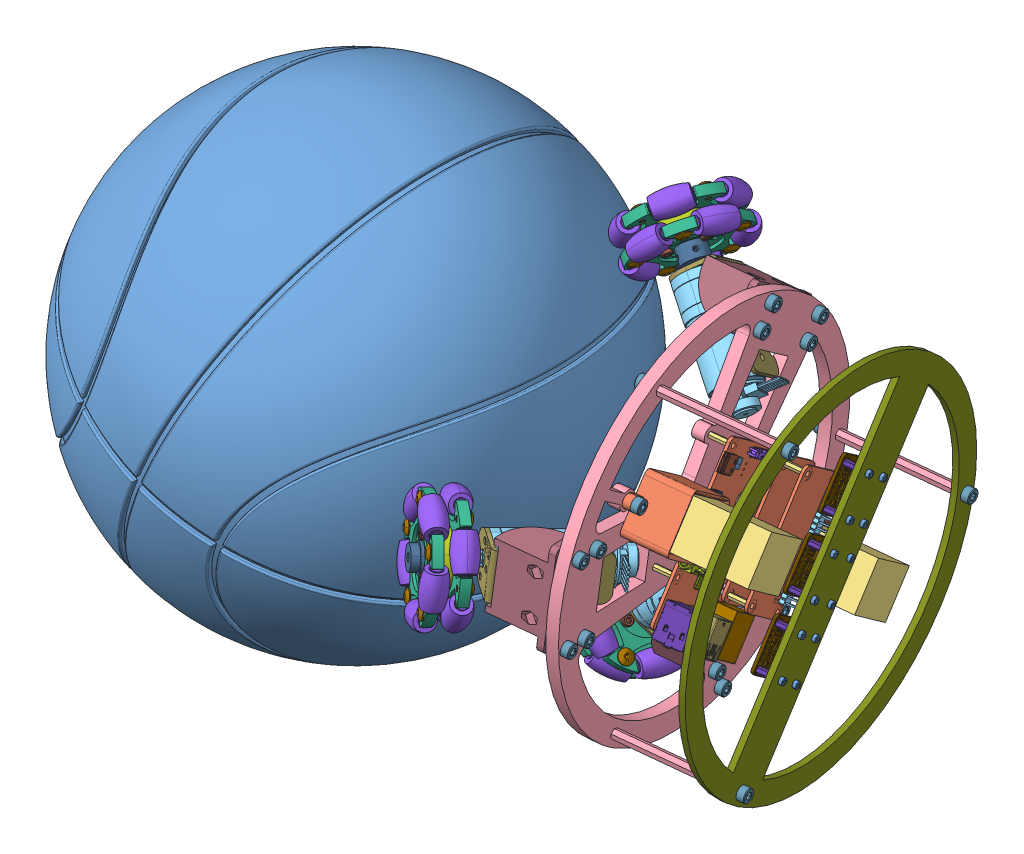
SolidWorks assembly FullAssembly, configuration Default. Lengths in mm.
Overall size (421.56 325.38 301.94).
211 component instances, 40 part files, 36 mates.
Components (placement in the parent):
- basketball-1: basketball [Default] at (262.8236 329.342 181.7922) x (0.927184 -0.374607 0) z (0 0 1) size (249.95 249.95 250.98)
- PiAssembly-1: PiAssembly [Default] at (395.3166 293.6839 90.7968) x (0.056245 -0.796975 0.601388) z (0.155278 0.601995 0.783257) size (89.02 42.68 58.4)
  - Raspberry Pi 4 Model B-1: Raspberry Pi 4 Model B [Default] at (23.6028 37.8671 72.1656) size (88.99 19.9 58.4)
    - PCB, RPi4ModelB-1: PCB, RPi4ModelB [Default] at origin size (85 1.6 56)
    - Broadcom BCM2711B0 CPU, RPi4ModelB-1: Broadcom BCM2711B0 CPU, RPi4ModelB [Default] at (-13.25 0.8 -4.5) size (15 2.3 15)
    - 2.54 mm DUPONT MALE PIN HEADER, POE, 2X2, RPi4ModelB-1: 2.54 mm DUPONT MALE PIN HEADER, POE, 2X2, RPi4ModelB [Default] at (19 0.8 -18.5) size (5.08 11.3 5.08)
    - 2.54 mm DUPONT MALE PIN HEADER, IO, 2X20, RPi4ModelB-1: 2.54 mm DUPONT MALE PIN HEADER, IO, 2X20, RPi4ModelB [Default] at (-10 0.8 -24.5) size (50.8 11.3 5.08)
    - Camera Connector, RPi4ModelB-1: Camera Connector, RPi4ModelB [Default] at (4 0.8 16.5) x (0 0 -1) z (1 0 0) size (22.4 5.68 5.07)
    - Microphone Plug, RPi4ModelB-1: Microphone Plug, RPi4ModelB [Default] at (11.5 0.8 21.65) size (7.23 7.55 15)
    - Display Connector, RPi4ModelB-1: Display Connector, RPi4ModelB [Default] at (-38.5 0.8 0) x (0 0 1) z (-1 0 0) size (22.4 5.68 5.07)
    - Gigabit Ethernet Port, RPi4ModelB-1: Gigabit Ethernet Port, RPi4ModelB [Default] at (45.5 7.55 -17.75) x (0 0 -1) z (1 0 0) size (16.2 17.24 21.64)
    - Female Micro HDMI Connector, RPi4ModelB-2: Female Micro HDMI Connector, RPi4ModelB [Default] at (-3 0.8 27.3875) size (6.5 3.51 7.5)
    - Female Micro HDMI Connector, RPi4ModelB-3: Female Micro HDMI Connector, RPi4ModelB [Default] at (-16.5 0.8 27.3875) size (6.5 3.51 7.5)
    - Female USB Type C Connector, RPi4ModelB-1: Female USB Type C Connector, RPi4ModelB [Default] at (-31.3 0.8 26.5419) size (8.94 3.96 7.9)
    - 2X USB3.0 PORTS, RPi4ModelB-2: 2X USB3.0 PORTS, RPi4ModelB [Default] at (37.07 0.8 1) size (17.47 19.41 15.68)
    - 91D77 D9WHV 778K, 4 GB LPDDR4 SDRAM, RPi4ModelB-1: 91D77 D9WHV 778K, 4 GB LPDDR4 SDRAM, RPi4ModelB [Default] at (2.25 0.8 -4.5) size (10 0.8 14.5)
    - Cypress CYW43455 Wireless Module Cover, RPi4ModelB-1: Cypress CYW43455 Wireless Module Cover, RPi4ModelB [Default] at (-30.5 0.8 -14.5) size (11 1.6 13)
    - SD Card Slot, RPi4ModelB-1: SD Card Slot, RPi4ModelB [Default] at (-35.3 -0.8 0) x (0 0 -1) z (-1 0 0) size (11.95 1.45 11.4)
    - VIA VL805 PCIe USB 3.0 controller, RPi4ModelB-1: VIA VL805 PCIe USB 3.0 controller, RPi4ModelB [Default] at (17.5 0.8 4) size (8.8 0.8 8.8)
    - 2X USB2.0 PORTS, RPi4ModelB-1: 2X USB2.0 PORTS, RPi4ModelB [Default] at (37.065 0.65 19) size (17.87 19.16 15.33)
    - Broadcom BCM54213PE Gigabit Ethernet Transceiver, RPi4ModelB-1: Broadcom BCM54213PE Gigabit Ethernet Transceiver, RPi4ModelB [Default] at (16.5 0.8 -10) size (6.8 1 6.8)
    - MxL7704 Universal PMIC, RPi4ModelB-1: MxL7704 Universal PMIC, RPi4ModelB [Default] at (-32.5 0.8 16) size (5.4 0.8 5.4)
  - Pi Motor Hat-1: Pi Motor Hat [Default] at (13.5778 60.0571 59.1906) size (65 1.5 30)
  - Pi Motor Hat-2: Pi Motor Hat [Default] at (13.5778 48.6571 59.1906) size (65 1.5 30)
  - PiStandoff-1: PiStandoff [Default] at (42.6028 50.0571 47.6656) x (0.096997 0 0.995285) z (-0.995285 0 0.096997) size (3.12 10 2.7)
  - PiStandoff-2: PiStandoff [Default] at (-15.3972 38.6571 47.6656) size (3.12 10 2.7)
  - PiStandoff-3: PiStandoff [Default] at (-15.4472 50.0571 47.6656) x (-0.525395 0 0.850858) z (-0.850858 0 -0.525395) size (3.12 10 2.7)
  - PiStandoff-4: PiStandoff [Default] at (42.6028 38.6571 47.6656) size (3.12 10 2.7)
  - PiStandoff-5: PiStandoff [Default] at (42.6028 50.0571 70.7156) x (0.1639 0 0.986477) z (-0.986477 0 0.1639) size (3.12 10 2.7)
  - PiStandoff-6: PiStandoff [Default] at (-15.4472 50.0571 70.7156) x (-0.245329 0 -0.96944) z (0.96944 0 -0.245329) size (3.12 10 2.7)
  - 2.54 mm DUPONT MALE PIN HEADER, IO, 2X20, RPi4ModelB-1: 2.54 mm DUPONT MALE PIN HEADER, IO, 2X20, RPi4ModelB [Default] at (13.6028 50.0571 47.6656) size (50.8 11.3 5.08)
  - 2.54 mm DUPONT MALE PIN HEADER, IO, 2X20, RPi4ModelB-2: 2.54 mm DUPONT MALE PIN HEADER, IO, 2X20, RPi4ModelB [Default] at (13.6028 61.4571 47.6656) size (50.8 11.3 5.08)
  - PiStandoff-7: PiStandoff [Default] at (42.6028 27.0771 47.6656) x (0.455658 0 0.890155) z (-0.890155 0 0.455658) size (3.12 10 2.7)
  - PiStandoff-8: PiStandoff [Default] at (-15.3972 27.0771 47.6656) x (-0.990783 0 0.135462) z (-0.135462 0 -0.990783) size (3.12 10 2.7)
  - PiStandoff-9: PiStandoff [Default] at (42.6028 27.0771 96.6656) x (0.096997 0 0.995285) z (-0.995285 0 0.096997) size (3.12 10 2.7)
  - PiStandoff-10: PiStandoff [Default] at (-15.3972 27.0771 96.6656) x (0.096997 0 0.995285) z (-0.995285 0 0.096997) size (3.12 10 2.7)
- BasePlate-1: BasePlate [Default] at (428.0251 321.0796 155.392) x (-0.155278 -0.601995 -0.783257) z (0.056245 -0.796975 0.601388) size (200 6.35 200)
- MotorAssembly-1: MotorAssembly [Default] at (403.3898 268.0903 115.0409) x (-0.126349 0.389203 -0.912445) z (-0.772599 -0.615538 -0.155574) size (87.54 86.92 94.1)
  - 25d-metal-gearmotor-20.4-encoder-1: 25d-metal-gearmotor-20.4-encoder [Default] at (-50.1822 -0.1991 13.7812) size (25 32.85 74)
  - WheelAsm-1: WheelAsm [Default] at (-21.6001 -5.321 -11.7274) x (0.801126 0.598496 0) z (0 0 1) size (63.86 60.79 27.6)
    - WheelAsm.STEP-1: WheelAsm.STEP [Default] at origin size (63.86 60.79 27.6)
      - WheelBase.STEP-1: WheelBase.STEP [Default] at (4.9023 2.731 55.3836) x (1 0 0) z (0 -1 0) size (56.86 5 54.96)
      - BasePlacer.STEP-1: BasePlacer.STEP [Default] at (4.9023 2.731 58.8836) x (1 0 0) z (0 -1 0) size (28 10 28)
      - RubberWheel.STEP-1: RubberWheel.STEP [Default] at (4.9023 26.7901 57.8836) x (1 0 0) z (0 -0.999594 -0.028494) size (19 12.5 12.5)
      - RubberWheel.STEP-2: RubberWheel.STEP [Default] at (-17.9792 10.1657 57.8836) x (0.309017 0.951057 0) z (0.95067 -0.308892 -0.028494) size (19 12.5 12.5)
      - RubberWheel.STEP-3: RubberWheel.STEP [Default] at (-9.2392 -16.7332 57.8836) x (-0.809017 0.587785 0) z (0.587547 0.808689 -0.028494) size (19 12.5 12.5)
      - RubberWheel.STEP-4: RubberWheel.STEP [Default] at (19.0439 -16.7332 57.8836) x (-0.809017 -0.587785 0) z (-0.587547 0.808689 -0.028494) size (19 12.5 12.5)
      - RubberWheel.STEP-5: RubberWheel.STEP [Default] at (27.7839 10.1657 57.8836) x (0.309017 -0.951057 0) z (-0.95067 -0.308892 -0.028494) size (19 12.5 12.5)
      - Rivet.STEP-1: Rivet.STEP [Default] at (4.9023 -21.269 54.8836) x (1 0 0) z (0 1 0) size (7.46 6.8 7.46)
      - Rivet.STEP-2: Rivet.STEP [Default] at (27.7277 -4.6854 54.8836) x (0.309017 0.951057 0) z (-0.951057 0.309017 0) size (7.46 6.8 7.46)
      - Rivet.STEP-3: Rivet.STEP [Default] at (19.0092 22.1474 54.8836) x (-0.809017 0.587785 0) z (-0.587785 -0.809017 0) size (7.46 6.8 7.46)
      - Rivet.STEP-4: Rivet.STEP [Default] at (-9.2045 22.1474 54.8836) x (-0.809017 -0.587785 0) z (0.587785 -0.809017 0) size (7.46 6.8 7.46)
      - Rivet.STEP-5: Rivet.STEP [Default] at (-17.923 -4.6854 54.8836) x (0.309017 -0.951057 0) z (0.951057 0.309017 0) size (7.46 6.8 7.46)
      - WheelBase.STEP-2: WheelBase.STEP [Default] at (4.9023 2.731 67.3836) x (-1 0 0) z (0 1 0) size (56.86 5 54.96)
      - RubberWheel.STEP-6: RubberWheel.STEP [Default] at (4.9023 -21.3281 69.8836) size (19 12.5 12.5)
      - RubberWheel.STEP-7: RubberWheel.STEP [Default] at (27.7839 -4.7037 69.8836) x (0.309017 0.951057 0) z (0 0 1) size (19 12.5 12.5)
      - RubberWheel.STEP-8: RubberWheel.STEP [Default] at (19.0439 22.1953 69.8836) x (-0.809017 0.587785 0) z (0 0 1) size (19 12.5 12.5)
      - RubberWheel.STEP-9: RubberWheel.STEP [Default] at (-9.2392 22.1953 69.8836) x (-0.809017 -0.587785 0) z (0 0 1) size (19 12.5 12.5)
      - RubberWheel.STEP-10: RubberWheel.STEP [Default] at (-17.9792 -4.7037 69.8836) x (0.309017 -0.951057 0) z (0 0 1) size (19 12.5 12.5)
      - Rivet.STEP-6: Rivet.STEP [Default] at (-9.2045 -16.6854 72.8836) x (-0.985624 0.168955 0) z (0.168955 0.985624 0) size (7.46 6.8 7.46)
      - Rivet.STEP-7: Rivet.STEP [Default] at (19.0092 -16.6854 72.8836) x (-0.46526 -0.885174 0) z (-0.885174 0.46526 0) size (7.46 6.8 7.46)
      - Rivet.STEP-8: Rivet.STEP [Default] at (27.7277 10.1474 72.8836) x (0.698077 -0.716022 0) z (-0.716022 -0.698077 0) size (7.46 6.8 7.46)
      - Rivet.STEP-9: Rivet.STEP [Default] at (4.9023 26.731 72.8836) x (0.896695 0.442648 0) z (0.442648 -0.896695 0) size (7.46 6.8 7.46)
      - Rivet.STEP-10: Rivet.STEP [Default] at (-17.923 10.1474 72.8836) x (-0.143889 0.989594 0) z (0.989594 0.143889 0) size (7.46 6.8 7.46)
      - ShaftConnector.STEP-1: ShaftConnector.STEP [Default] at (4.9023 2.731 48.8836) x (1 0 0) z (0 -1 0) size (14.01 27.6 14.01)
      - M3HexNut.STEP-1: M3HexNut.STEP [Default] at (13.9956 7.981 72.8836) x (1 0 0) z (0 0 -1) size (5 5 5)
      - M3HexNut.STEP-2: M3HexNut.STEP [Default] at (-4.1909 7.981 72.8836) x (-0.5 0.866025 0) z (0 0 -1) size (5 5 5)
      - M3HexNut.STEP-3: M3HexNut.STEP [Default] at (4.9023 -7.769 72.8836) x (-0.5 -0.866025 0) z (0 0 -1) size (5 5 5)
      - M3HexNut.STEP-4: M3HexNut.STEP [Default] at (4.9023 -7.769 54.8836) size (5 5 5)
      - M3HexNut.STEP-5: M3HexNut.STEP [Default] at (13.9956 7.981 54.8836) x (-0.5 0.866025 0) z (0 0 1) size (5 5 5)
      - M3HexNut.STEP-6: M3HexNut.STEP [Default] at (-4.1909 7.981 54.8836) x (-0.5 -0.866025 0) z (0 0 1) size (5 5 5)
  - pololu-25d-mm-metal-gearmotor-bracket-1: pololu-25d-mm-metal-gearmotor-bracket [Default] at (-20.3072 0.8009 19.6562) x (-1 0 0) z (0 0 1) size (25 27 52)
  - MotorMount-1: MotorMount [Default] at (-1.8072 14.6545 14.1971) x (0 0.707107 0.707107) z (0 -0.707107 0.707107) size (24 50 30)
  - M4x6-1: M4x6 [Default] at (-40.5572 28.337 -7.9707) x (0 -0.707107 0.707107) z (-0.996625 0.05805 0.05805) size (12.15 7 7)
  - M4x6-2: M4x6 [Default] at (-40.5572 36.8223 0.5146) x (0 -0.707107 0.707107) z (-0.996625 0.05805 0.05805) size (12.15 7 7)
  - M3x4-3: M3x4 [Default] at (-8.4572 11.3009 18.2812) x (0 1 0) z (-0.998192 0 -0.0601) size (7 5.5 5.5)
  - M3x4-4: M3x4 [Default] at (-30.1572 11.3009 18.2812) x (0 1 0) z (-0.546944 0 0.837169) size (7 5.5 5.5)
  - M4x6-3: M4x6 [Default] at (1.9428 28.337 -7.9707) x (0 -0.707107 0.707107) z (-0.996625 0.05805 0.05805) size (12.15 7 7)
  - M4x6-4: M4x6 [Default] at (1.9428 36.8223 0.5146) x (0 -0.707107 0.707107) z (-0.996625 0.05805 0.05805) size (12.15 7 7)
- MotorAssembly-2: MotorAssembly [Default] at (412.1642 386.5359 132.8779) x (0.155278 0.601995 0.783257) z (-0.737168 0.598426 -0.313797) size (87.54 86.92 94.1)
  - 25d-metal-gearmotor-20.4-encoder-1: 25d-metal-gearmotor-20.4-encoder [Default] at (-50.1822 -0.1991 13.7812) size (25 32.85 74)
  - WheelAsm-1: WheelAsm [Default] at (-21.6001 -5.321 -11.7274) x (0.801126 0.598496 0) z (0 0 1) size (63.86 60.79 27.6)
    - WheelAsm.STEP-1: WheelAsm.STEP [Default] at origin size (63.86 60.79 27.6)
      - WheelBase.STEP-1: WheelBase.STEP [Default] at (4.9023 2.731 55.3836) x (1 0 0) z (0 -1 0) size (56.86 5 54.96)
      - BasePlacer.STEP-1: BasePlacer.STEP [Default] at (4.9023 2.731 58.8836) x (1 0 0) z (0 -1 0) size (28 10 28)
      - RubberWheel.STEP-1: RubberWheel.STEP [Default] at (4.9023 26.7901 57.8836) x (1 0 0) z (0 -0.999594 -0.028494) size (19 12.5 12.5)
      - RubberWheel.STEP-2: RubberWheel.STEP [Default] at (-17.9792 10.1657 57.8836) x (0.309017 0.951057 0) z (0.95067 -0.308892 -0.028494) size (19 12.5 12.5)
      - RubberWheel.STEP-3: RubberWheel.STEP [Default] at (-9.2392 -16.7332 57.8836) x (-0.809017 0.587785 0) z (0.587547 0.808689 -0.028494) size (19 12.5 12.5)
      - RubberWheel.STEP-4: RubberWheel.STEP [Default] at (19.0439 -16.7332 57.8836) x (-0.809017 -0.587785 0) z (-0.587547 0.808689 -0.028494) size (19 12.5 12.5)
      - RubberWheel.STEP-5: RubberWheel.STEP [Default] at (27.7839 10.1657 57.8836) x (0.309017 -0.951057 0) z (-0.95067 -0.308892 -0.028494) size (19 12.5 12.5)
      - Rivet.STEP-1: Rivet.STEP [Default] at (4.9023 -21.269 54.8836) x (1 0 0) z (0 1 0) size (7.46 6.8 7.46)
      - Rivet.STEP-2: Rivet.STEP [Default] at (27.7277 -4.6854 54.8836) x (0.309017 0.951057 0) z (-0.951057 0.309017 0) size (7.46 6.8 7.46)
      - Rivet.STEP-3: Rivet.STEP [Default] at (19.0092 22.1474 54.8836) x (-0.809017 0.587785 0) z (-0.587785 -0.809017 0) size (7.46 6.8 7.46)
      - Rivet.STEP-4: Rivet.STEP [Default] at (-9.2045 22.1474 54.8836) x (-0.809017 -0.587785 0) z (0.587785 -0.809017 0) size (7.46 6.8 7.46)
      - Rivet.STEP-5: Rivet.STEP [Default] at (-17.923 -4.6854 54.8836) x (0.309017 -0.951057 0) z (0.951057 0.309017 0) size (7.46 6.8 7.46)
      - WheelBase.STEP-2: WheelBase.STEP [Default] at (4.9023 2.731 67.3836) x (-1 0 0) z (0 1 0) size (56.86 5 54.96)
      - RubberWheel.STEP-6: RubberWheel.STEP [Default] at (4.9023 -21.3281 69.8836) size (19 12.5 12.5)
      - RubberWheel.STEP-7: RubberWheel.STEP [Default] at (27.7839 -4.7037 69.8836) x (0.309017 0.951057 0) z (0 0 1) size (19 12.5 12.5)
      - RubberWheel.STEP-8: RubberWheel.STEP [Default] at (19.0439 22.1953 69.8836) x (-0.809017 0.587785 0) z (0 0 1) size (19 12.5 12.5)
      - RubberWheel.STEP-9: RubberWheel.STEP [Default] at (-9.2392 22.1953 69.8836) x (-0.809017 -0.587785 0) z (0 0 1) size (19 12.5 12.5)
      - RubberWheel.STEP-10: RubberWheel.STEP [Default] at (-17.9792 -4.7037 69.8836) x (0.309017 -0.951057 0) z (0 0 1) size (19 12.5 12.5)
      - Rivet.STEP-6: Rivet.STEP [Default] at (-9.2045 -16.6854 72.8836) x (-0.985624 0.168955 0) z (0.168955 0.985624 0) size (7.46 6.8 7.46)
      - Rivet.STEP-7: Rivet.STEP [Default] at (19.0092 -16.6854 72.8836) x (-0.46526 -0.885174 0) z (-0.885174 0.46526 0) size (7.46 6.8 7.46)
      - Rivet.STEP-8: Rivet.STEP [Default] at (27.7277 10.1474 72.8836) x (0.698077 -0.716022 0) z (-0.716022 -0.698077 0) size (7.46 6.8 7.46)
      - Rivet.STEP-9: Rivet.STEP [Default] at (4.9023 26.731 72.8836) x (0.896695 0.442648 0) z (0.442648 -0.896695 0) size (7.46 6.8 7.46)
      - Rivet.STEP-10: Rivet.STEP [Default] at (-17.923 10.1474 72.8836) x (-0.143889 0.989594 0) z (0.989594 0.143889 0) size (7.46 6.8 7.46)
      - ShaftConnector.STEP-1: ShaftConnector.STEP [Default] at (4.9023 2.731 48.8836) x (1 0 0) z (0 -1 0) size (14.01 27.6 14.01)
      - M3HexNut.STEP-1: M3HexNut.STEP [Default] at (13.9956 7.981 72.8836) x (1 0 0) z (0 0 -1) size (5 5 5)
      - M3HexNut.STEP-2: M3HexNut.STEP [Default] at (-4.1909 7.981 72.8836) x (-0.5 0.866025 0) z (0 0 -1) size (5 5 5)
      - M3HexNut.STEP-3: M3HexNut.STEP [Default] at (4.9023 -7.769 72.8836) x (-0.5 -0.866025 0) z (0 0 -1) size (5 5 5)
      - M3HexNut.STEP-4: M3HexNut.STEP [Default] at (4.9023 -7.769 54.8836) size (5 5 5)
      - M3HexNut.STEP-5: M3HexNut.STEP [Default] at (13.9956 7.981 54.8836) x (-0.5 0.866025 0) z (0 0 1) size (5 5 5)
      - M3HexNut.STEP-6: M3HexNut.STEP [Default] at (-4.1909 7.981 54.8836) x (-0.5 -0.866025 0) z (0 0 1) size (5 5 5)
  - pololu-25d-mm-metal-gearmotor-bracket-1: pololu-25d-mm-metal-gearmotor-bracket [Default] at (-20.3072 0.8009 19.6562) x (-1 0 0) z (0 0 1) size (25 27 52)
  - MotorMount-1: MotorMount [Default] at (-1.8072 14.6545 14.1971) x (0 0.707107 0.707107) z (0 -0.707107 0.707107) size (24 50 30)
  - M4x6-1: M4x6 [Default] at (-40.5572 28.337 -7.9707) x (0 -0.707107 0.707107) z (-0.996625 0.05805 0.05805) size (12.15 7 7)
  - M4x6-2: M4x6 [Default] at (-40.5572 36.8223 0.5146) x (0 -0.707107 0.707107) z (-0.996625 0.05805 0.05805) size (12.15 7 7)
  - M3x4-3: M3x4 [Default] at (-8.4572 11.3009 18.2812) x (0 1 0) z (-0.998192 0 -0.0601) size (7 5.5 5.5)
  - M3x4-4: M3x4 [Default] at (-30.1572 11.3009 18.2812) x (0 1 0) z (-0.546944 0 0.837169) size (7 5.5 5.5)
  - M4x6-3: M4x6 [Default] at (1.9428 28.337 -7.9707) x (0 -0.707107 0.707107) z (-0.996625 0.05805 0.05805) size (12.15 7 7)
  - M4x6-4: M4x6 [Default] at (1.9428 36.8223 0.5146) x (0 -0.707107 0.707107) z (-0.996625 0.05805 0.05805) size (12.15 7 7)
- MotorAssembly-3: MotorAssembly [Default] at (423.1824 310.8802 225.5027) x (-0.028929 -0.991198 0.129189) z (-0.582424 0.121751 0.803716) size (87.54 86.92 94.1)
  - 25d-metal-gearmotor-20.4-encoder-1: 25d-metal-gearmotor-20.4-encoder [Default] at (-50.1822 -0.1991 13.7812) size (25 32.85 74)
  - WheelAsm-1: WheelAsm [Default] at (-21.6001 -5.321 -11.7274) x (0.801126 0.598496 0) z (0 0 1) size (63.86 60.79 27.6)
    - WheelAsm.STEP-1: WheelAsm.STEP [Default] at origin size (63.86 60.79 27.6)
      - WheelBase.STEP-1: WheelBase.STEP [Default] at (4.9023 2.731 55.3836) x (1 0 0) z (0 -1 0) size (56.86 5 54.96)
      - BasePlacer.STEP-1: BasePlacer.STEP [Default] at (4.9023 2.731 58.8836) x (1 0 0) z (0 -1 0) size (28 10 28)
      - RubberWheel.STEP-1: RubberWheel.STEP [Default] at (4.9023 26.7901 57.8836) x (1 0 0) z (0 -0.999594 -0.028494) size (19 12.5 12.5)
      - RubberWheel.STEP-2: RubberWheel.STEP [Default] at (-17.9792 10.1657 57.8836) x (0.309017 0.951057 0) z (0.95067 -0.308892 -0.028494) size (19 12.5 12.5)
      - RubberWheel.STEP-3: RubberWheel.STEP [Default] at (-9.2392 -16.7332 57.8836) x (-0.809017 0.587785 0) z (0.587547 0.808689 -0.028494) size (19 12.5 12.5)
      - RubberWheel.STEP-4: RubberWheel.STEP [Default] at (19.0439 -16.7332 57.8836) x (-0.809017 -0.587785 0) z (-0.587547 0.808689 -0.028494) size (19 12.5 12.5)
      - RubberWheel.STEP-5: RubberWheel.STEP [Default] at (27.7839 10.1657 57.8836) x (0.309017 -0.951057 0) z (-0.95067 -0.308892 -0.028494) size (19 12.5 12.5)
      - Rivet.STEP-1: Rivet.STEP [Default] at (4.9023 -21.269 54.8836) x (1 0 0) z (0 1 0) size (7.46 6.8 7.46)
      - Rivet.STEP-2: Rivet.STEP [Default] at (27.7277 -4.6854 54.8836) x (0.309017 0.951057 0) z (-0.951057 0.309017 0) size (7.46 6.8 7.46)
      - Rivet.STEP-3: Rivet.STEP [Default] at (19.0092 22.1474 54.8836) x (-0.809017 0.587785 0) z (-0.587785 -0.809017 0) size (7.46 6.8 7.46)
      - Rivet.STEP-4: Rivet.STEP [Default] at (-9.2045 22.1474 54.8836) x (-0.809017 -0.587785 0) z (0.587785 -0.809017 0) size (7.46 6.8 7.46)
      - Rivet.STEP-5: Rivet.STEP [Default] at (-17.923 -4.6854 54.8836) x (0.309017 -0.951057 0) z (0.951057 0.309017 0) size (7.46 6.8 7.46)
      - WheelBase.STEP-2: WheelBase.STEP [Default] at (4.9023 2.731 67.3836) x (-1 0 0) z (0 1 0) size (56.86 5 54.96)
      - RubberWheel.STEP-6: RubberWheel.STEP [Default] at (4.9023 -21.3281 69.8836) size (19 12.5 12.5)
      - RubberWheel.STEP-7: RubberWheel.STEP [Default] at (27.7839 -4.7037 69.8836) x (0.309017 0.951057 0) z (0 0 1) size (19 12.5 12.5)
      - RubberWheel.STEP-8: RubberWheel.STEP [Default] at (19.0439 22.1953 69.8836) x (-0.809017 0.587785 0) z (0 0 1) size (19 12.5 12.5)
      - RubberWheel.STEP-9: RubberWheel.STEP [Default] at (-9.2392 22.1953 69.8836) x (-0.809017 -0.587785 0) z (0 0 1) size (19 12.5 12.5)
      - RubberWheel.STEP-10: RubberWheel.STEP [Default] at (-17.9792 -4.7037 69.8836) x (0.309017 -0.951057 0) z (0 0 1) size (19 12.5 12.5)
      - Rivet.STEP-6: Rivet.STEP [Default] at (-9.2045 -16.6854 72.8836) x (-0.985624 0.168955 0) z (0.168955 0.985624 0) size (7.46 6.8 7.46)
      - Rivet.STEP-7: Rivet.STEP [Default] at (19.0092 -16.6854 72.8836) x (-0.46526 -0.885174 0) z (-0.885174 0.46526 0) size (7.46 6.8 7.46)
      - Rivet.STEP-8: Rivet.STEP [Default] at (27.7277 10.1474 72.8836) x (0.698077 -0.716022 0) z (-0.716022 -0.698077 0) size (7.46 6.8 7.46)
      - Rivet.STEP-9: Rivet.STEP [Default] at (4.9023 26.731 72.8836) x (0.896695 0.442648 0) z (0.442648 -0.896695 0) size (7.46 6.8 7.46)
      - Rivet.STEP-10: Rivet.STEP [Default] at (-17.923 10.1474 72.8836) x (-0.143889 0.989594 0) z (0.989594 0.143889 0) size (7.46 6.8 7.46)
      - ShaftConnector.STEP-1: ShaftConnector.STEP [Default] at (4.9023 2.731 48.8836) x (1 0 0) z (0 -1 0) size (14.01 27.6 14.01)
      - M3HexNut.STEP-1: M3HexNut.STEP [Default] at (13.9956 7.981 72.8836) x (1 0 0) z (0 0 -1) size (5 5 5)
      - M3HexNut.STEP-2: M3HexNut.STEP [Default] at (-4.1909 7.981 72.8836) x (-0.5 0.866025 0) z (0 0 -1) size (5 5 5)
      - M3HexNut.STEP-3: M3HexNut.STEP [Default] at (4.9023 -7.769 72.8836) x (-0.5 -0.866025 0) z (0 0 -1) size (5 5 5)
      - M3HexNut.STEP-4: M3HexNut.STEP [Default] at (4.9023 -7.769 54.8836) size (5 5 5)
      - M3HexNut.STEP-5: M3HexNut.STEP [Default] at (13.9956 7.981 54.8836) x (-0.5 0.866025 0) z (0 0 1) size (5 5 5)
      - M3HexNut.STEP-6: M3HexNut.STEP [Default] at (-4.1909 7.981 54.8836) x (-0.5 -0.866025 0) z (0 0 1) size (5 5 5)
  - pololu-25d-mm-metal-gearmotor-bracket-1: pololu-25d-mm-metal-gearmotor-bracket [Default] at (-20.3072 0.8009 19.6562) x (-1 0 0) z (0 0 1) size (25 27 52)
  - MotorMount-1: MotorMount [Default] at (-1.8072 14.6545 14.1971) x (0 0.707107 0.707107) z (0 -0.707107 0.707107) size (24 50 30)
  - M4x6-1: M4x6 [Default] at (-40.5572 28.337 -7.9707) x (0 -0.707107 0.707107) z (-0.996625 0.05805 0.05805) size (12.15 7 7)
  - M4x6-2: M4x6 [Default] at (-40.5572 36.8223 0.5146) x (0 -0.707107 0.707107) z (-0.996625 0.05805 0.05805) size (12.15 7 7)
  - M3x4-3: M3x4 [Default] at (-8.4572 11.3009 18.2812) x (0 1 0) z (-0.998192 0 -0.0601) size (7 5.5 5.5)
  - M3x4-4: M3x4 [Default] at (-30.1572 11.3009 18.2812) x (0 1 0) z (-0.546944 0 0.837169) size (7 5.5 5.5)
  - M4x6-3: M4x6 [Default] at (1.9428 28.337 -7.9707) x (0 -0.707107 0.707107) z (-0.996625 0.05805 0.05805) size (12.15 7 7)
  - M4x6-4: M4x6 [Default] at (1.9428 36.8223 0.5146) x (0 -0.707107 0.707107) z (-0.996625 0.05805 0.05805) size (12.15 7 7)
- TopAssembly-1: TopAssembly [Default] at (362.6924 300.9635 -5.5567) x (0.056245 -0.796975 0.601388) z (0.155278 0.601995 0.783257) size (200 16.92 200)
  - TopPlate-1: TopPlate [Default] at (84.4352 104.4259 148.3187) size (200 3.17 200)
  - SensorStandoff-1: SensorStandoff [Default] at (38.9552 96.4259 154.6687) size (3.46 8 3.03)
  - SensorStandoff-2: SensorStandoff [Default] at (38.9552 104.4259 141.9687) x (-0.837169 0 -0.546944) z (-0.546944 0 0.837169) size (3.46 8 3.03)
  - SensorStandoff-3: SensorStandoff [Default] at (59.2752 96.4259 154.6687) size (3.46 8 3.03)
  - SensorStandoff-4: SensorStandoff [Default] at (59.2752 96.4259 141.9687) size (3.46 8 3.03)
  - SensorStandoff-5: SensorStandoff [Default] at (74.2752 96.4259 140.6987) size (3.46 8 3.03)
  - SensorStandoff-6: SensorStandoff [Default] at (74.2752 96.4259 155.9387) size (3.46 8 3.03)
  - SensorStandoff-7: SensorStandoff [Default] at (94.5952 96.4259 140.6987) size (3.46 8 3.03)
  - SensorStandoff-8: SensorStandoff [Default] at (94.5952 96.4259 155.9387) size (3.46 8 3.03)
  - SensorStandoff-9: SensorStandoff [Default] at (109.5952 96.4259 141.9687) size (3.46 8 3.03)
  - SensorStandoff-10: SensorStandoff [Default] at (109.5952 96.4259 154.6687) size (3.46 8 3.03)
  - SensorStandoff-11: SensorStandoff [Default] at (129.9152 96.4259 141.9687) size (3.46 8 3.03)
  - SensorStandoff-12: SensorStandoff [Default] at (129.9152 96.4259 154.6687) size (3.46 8 3.03)
  - Adafruit_BNO055-1: Adafruit_BNO055 [Default] at (70.4652 94.7259 158.4787) size (26.67 4.2 20.32)
  - Adafruit_BNO055-2: Adafruit_BNO055 [Default] at (105.7852 94.7259 157.2087) size (26.67 4.2 20.32)
  - Adafruit_BNO055-3: Adafruit_BNO055 [Default] at (35.1452 94.7259 157.2087) size (26.67 4.2 20.32)
  - M4x6-3: M4x6 [Default] at (178.4352 111.6009 148.3187) x (0 -1 0) z (-0.901546 0 0.432684) size (12.15 7 7)
  - M2x0.8_NoThread-1: M2x0.8_NoThread [Default] at (94.5952 107.6009 140.6987) size (3.62 10 3.62)
  - M2x0.8_NoThread-2: M2x0.8_NoThread [Default] at (94.5952 107.6009 155.9387) size (3.62 10 3.62)
  - M2x0.8_NoThread-3: M2x0.8_NoThread [Default] at (129.9152 107.6009 141.9687) size (3.62 10 3.62)
  - M2x0.8_NoThread-4: M2x0.8_NoThread [Default] at (109.5952 107.6009 141.9687) size (3.62 10 3.62)
  - M2x0.8_NoThread-5: M2x0.8_NoThread [Default] at (109.5952 107.6009 154.6687) size (3.62 10 3.62)
  - M2x0.8_NoThread-6: M2x0.8_NoThread [Default] at (129.9152 107.6009 154.6687) size (3.62 10 3.62)
  - M2x0.8_NoThread-7: M2x0.8_NoThread [Default] at (38.9552 107.6009 141.9687) size (3.62 10 3.62)
  - M2x0.8_NoThread-8: M2x0.8_NoThread [Default] at (38.9552 107.6009 154.6687) size (3.62 10 3.62)
  - M2x0.8_NoThread-9: M2x0.8_NoThread [Default] at (59.2752 107.6009 141.9687) size (3.62 10 3.62)
  - M2x0.8_NoThread-10: M2x0.8_NoThread [Default] at (74.2752 107.6009 140.6987) size (3.62 10 3.62)
  - M2x0.8_NoThread-11: M2x0.8_NoThread [Default] at (59.2752 107.6009 154.6687) size (3.62 10 3.62)
  - M2x0.8_NoThread-12: M2x0.8_NoThread [Default] at (74.2752 107.6009 155.9387) size (3.62 10 3.62)
  - M4x6-7: M4x6 [Default] at (37.4352 111.6009 66.9123) x (0 -1 0) z (-0.901546 0 0.432684) size (12.15 7 7)
  - M4x6-8: M4x6 [Default] at (37.4352 111.6009 229.7251) x (0 -1 0) z (-0.901546 0 0.432684) size (12.15 7 7)
- M4x6-20: M4x6 [Default] at (429.3671 246.3612 212.5529) x (0.986268 -0.049328 -0.157612) z (0.153704 -0.074952 0.98527) size (12.15 7 7)
- LiPo Battery Assembly-1: LiPo Battery Assembly [Default] at (414.755 337.1936 109.9596) x (-0.155278 -0.601995 -0.783257) z (0.056245 -0.796975 0.601388) size (50 66.15 30)
  - LiPo Battery Holder-1: LiPo Battery Holder [Default] at (20.5548 15.072 40.9114) size (50 24 30)
  - LiPo Battery-1: LiPo Battery [Default] at (20.5548 45.072 28.4114) x (0 -1 0) z (-1 0 0) size (60 25 28)
  - M4x6-1: M4x6 [Default] at (-0.9452 21.072 40.9114) x (0 -1 0) z (0 0 1) size (12.15 7 7)
  - M4x6-2: M4x6 [Default] at (42.0548 21.072 40.9114) x (0 -1 0) z (0 0 1) size (12.15 7 7)
- LiPo Battery Assembly-2: LiPo Battery Assembly [Default] at (428.0357 305.6287 202.9434) x (0.155278 0.601995 0.783257) z (-0.056245 0.796975 -0.601388) size (50 66.15 30)
  - LiPo Battery Holder-1: LiPo Battery Holder [Default] at (20.5548 15.072 40.9114) size (50 24 30)
  - LiPo Battery-1: LiPo Battery [Default] at (20.5548 45.072 28.4114) x (0 -1 0) z (-1 0 0) size (60 25 28)
  - M4x6-1: M4x6 [Default] at (-0.9452 21.072 40.9114) x (0 -1 0) z (0 0 1) size (12.15 7 7)
  - M4x6-2: M4x6 [Default] at (42.0548 21.072 40.9114) x (0 -1 0) z (0 0 1) size (12.15 7 7)
- MiddlePlateStandoff-7: MiddlePlateStandoff [Default] at (498.7511 242.891 201.4649) x (0.073001 0.986268 0.14814) z (0.14814 -0.157612 0.976326) size (5.19 60 4.63)
- MiddlePlateStandoff-8: MiddlePlateStandoff [Default] at (478.1799 306.2583 52.9071) x (0.073001 0.986268 0.14814) z (0.14814 -0.157612 0.976326) size (5.19 60 4.63)
- MiddlePlateStandoff-9: MiddlePlateStandoff [Default] at (503.4611 404.2707 180.4314) x (0.073001 0.986268 0.14814) z (0.14814 -0.157612 0.976326) size (5.19 60 4.63)
- M4x6-21: M4x6 [Default] at (434.0771 407.7409 191.5194) x (0.986268 -0.049328 -0.157612) z (0.153704 -0.074952 0.98527) size (12.15 7 7)
- M4x6-22: M4x6 [Default] at (408.7959 309.7285 63.9951) x (0.986268 -0.049328 -0.157612) z (0.153704 -0.074952 0.98527) size (12.15 7 7)
Mates (geometry in assembly coordinates):
- Coincident6: coincident anti-aligned: plane of BasePlate-1 through (428.0251 321.0796 155.392) normal (-0.986268 0.049328 0.157612); plane of MotorAssembly-3/MotorMount-1 through (440.7262 347.6397 226.5573) normal (0.986268 -0.049328 -0.157612)
- Coincident7: coincident anti-aligned: plane of BasePlate-1 through (428.0251 321.0796 155.392) normal (-0.986268 0.049328 0.157612); plane of MotorAssembly-2/MotorMount-1 through (421.0894 370.3178 96.5809) normal (0.986268 -0.049328 -0.157612)
- Coincident8: coincident anti-aligned: plane of BasePlate-1 through (428.0251 321.0796 155.392) normal (-0.986268 0.049328 0.157612); plane of MotorAssembly-1/MotorMount-1 through (422.2598 245.2813 143.0378) normal (0.986268 -0.049328 -0.157612)
- Tangent6: tangent: sphere of basketball-1; circle of MotorAssembly-2/WheelAsm-1/WheelAsm.STEP-1/RubberWheel.STEP-3
- Tangent7: tangent: sphere of basketball-1; circle of MotorAssembly-3/WheelAsm-1/WheelAsm.STEP-1/RubberWheel.STEP-3
- Tangent8: tangent: sphere of basketball-1; circle of MotorAssembly-1/WheelAsm-1/WheelAsm.STEP-1/RubberWheel.STEP-3
- Concentric44: concentric anti-aligned: cylinder of BasePlate-1 through (427.454 246.4569 212.8586) axis (0.986268 -0.049328 -0.157612) radius 2.1; cylinder of M4x6-20 through (341.8797 250.7369 226.5339) axis (-0.986268 0.049328 0.157612) radius 3.5
- Coincident29: coincident anti-aligned: plane of BasePlate-1 through (428.0251 321.0796 155.392) normal (-0.986268 0.049328 0.157612); plane of M4x6-20 through (433.4323 248.1449 212.0544) normal (0.986268 -0.049328 -0.157612)
- Concentric48: concentric anti-aligned: cylinder of BasePlate-1 through (432.3568 407.6774 115.1063) axis (-0.986268 0.049328 0.157612) radius 2.1; cylinder of MotorAssembly-2/M4x6-4 through (523.7893 403.1045 100.4949) axis (0.986268 -0.049328 -0.157612) radius 3.5
- Concentric49: concentric anti-aligned: cylinder of BasePlate-1 through (425.7575 382.0927 81.8179) axis (-0.986268 0.049328 0.157612) radius 2.1; cylinder of MotorAssembly-2/M4x6-2 through (517.19 377.5197 67.2064) axis (0.986268 -0.049328 -0.157612) radius 3.5
- Concentric50: concentric anti-aligned: cylinder of BasePlate-1 through (450.0242 353.2548 242.6942) axis (-0.986268 0.049328 0.157612) radius 2.1; cylinder of MotorAssembly-3/M4x6-2 through (541.4567 348.6819 228.0828) axis (0.986268 -0.049328 -0.157612) radius 3.5
- Concentric51: concentric anti-aligned: cylinder of BasePlate-1 through (448.7947 311.1289 248.1848) axis (-0.986268 0.049328 0.157612) radius 2.1; cylinder of MotorAssembly-3/M4x6-4 through (540.2272 306.556 233.5733) axis (0.986268 -0.049328 -0.157612) radius 3.5
- Concentric52: concentric anti-aligned: cylinder of BasePlate-1 through (421.7123 243.4927 99.8824) axis (-0.986268 0.049328 0.157612) radius 2.1; cylinder of MotorAssembly-1/M4x6-4 through (513.1448 238.9198 85.271) axis (0.986268 -0.049328 -0.157612) radius 3.5
- Concentric53: concentric anti-aligned: cylinder of BasePlate-1 through (427.0821 226.9516 138.6614) axis (-0.986268 0.049328 0.157612) radius 2.1; cylinder of MotorAssembly-1/M4x6-2 through (518.5146 222.3786 124.0499) axis (0.986268 -0.049328 -0.157612) radius 3.5
- Concentric54: concentric aligned: cylinder of BasePlate-1 through (434.2879 320.7664 154.3912) axis (-0.986268 0.049328 0.157612) radius 100; cylinder of TopAssembly-1/TopPlate-1 through (496.5954 317.6501 144.4341) axis (-0.986268 0.049328 0.157612) radius 100
- Coincident35: coincident anti-aligned: plane of PiAssembly-1/PiStandoff-7 through (431.8195 287.0893 149.4843) normal (-0.986268 0.049328 0.157612); plane of BasePlate-1 through (434.2879 320.7664 154.3912) normal (0.986268 -0.049328 -0.157612)
- Concentric57: concentric aligned: circle of PiAssembly-1/PiStandoff-8; cylinder of BasePlate-1 through (418.5285 333.8155 116.2065) axis (0.986268 -0.049328 -0.157612) radius 1.35
- Concentric58: concentric anti-aligned: cylinder of PiAssembly-1/PiStandoff-9 through (449.2907 316.0938 186.2878) axis (-0.986268 0.049328 0.157612) radius 1.25; cylinder of BasePlate-1 through (429.3993 317.0886 189.4666) axis (0.986268 -0.049328 -0.157612) radius 1.35
- Coincident36: coincident anti-aligned: plane of BasePlate-1 through (434.2879 320.7664 154.3912) normal (0.986268 -0.049328 -0.157612); plane of LiPo Battery Assembly-1/LiPo Battery Holder-1 through (426.757 291.5696 116.4032) normal (-0.986268 0.049328 0.157612)
- Coincident37: coincident anti-aligned: plane of BasePlate-1 through (434.2879 320.7664 154.3912) normal (0.986268 -0.049328 -0.157612); plane of LiPo Battery Assembly-2/LiPo Battery Holder-1 through (441.8189 349.9631 192.3791) normal (-0.986268 0.049328 0.157612)
- Coincident38: coincident anti-aligned: plane of TopAssembly-1/TopPlate-1 through (493.464 317.8067 144.9345) normal (-0.986268 0.049328 0.157612); plane of MiddlePlateStandoff-7 through (498.7511 242.891 201.4649) normal (0.986268 -0.049328 -0.157612)
- Coincident39: coincident anti-aligned: plane of BasePlate-1 through (434.2879 320.7664 154.3912) normal (0.986268 -0.049328 -0.157612); plane of MiddlePlateStandoff-7 through (439.575 245.8507 210.9216) normal (-0.986268 0.049328 0.157612)
- Concentric71: concentric aligned: cylinder of BasePlate-1 through (427.454 246.4569 212.8586) axis (0.986268 -0.049328 -0.157612) radius 2.1; cylinder of MiddlePlateStandoff-7 through (439.575 245.8507 210.9216) axis (0.986268 -0.049328 -0.157612) radius 2
- Concentric72: concentric anti-aligned: cylinder of BasePlate-1 through (432.1641 407.8366 191.8251) axis (0.986268 -0.049328 -0.157612) radius 2.1; cylinder of M4x6-21 through (346.5897 412.1166 205.5004) axis (-0.986268 0.049328 0.157612) radius 3.5
- Coincident40: coincident anti-aligned: plane of BasePlate-1 through (428.0251 321.0796 155.392) normal (-0.986268 0.049328 0.157612); plane of M4x6-21 through (438.1424 409.5246 191.0209) normal (0.986268 -0.049328 -0.157612)
- Concentric73: concentric anti-aligned: cylinder of BasePlate-1 through (406.8829 309.8242 64.3008) axis (0.986268 -0.049328 -0.157612) radius 2.1; cylinder of M4x6-22 through (321.3085 314.1042 77.9762) axis (-0.986268 0.049328 0.157612) radius 3.5
- Coincident41: coincident anti-aligned: plane of BasePlate-1 through (428.0251 321.0796 155.392) normal (-0.986268 0.049328 0.157612); plane of M4x6-22 through (412.8612 311.5122 63.4966) normal (0.986268 -0.049328 -0.157612)
- Coincident42: coincident anti-aligned: plane of TopAssembly-1/TopPlate-1 through (493.464 317.8067 144.9345) normal (-0.986268 0.049328 0.157612); plane of MiddlePlateStandoff-9 through (503.4611 404.2707 180.4314) normal (0.986268 -0.049328 -0.157612)
- Coincident43: coincident anti-aligned: plane of BasePlate-1 through (434.2879 320.7664 154.3912) normal (0.986268 -0.049328 -0.157612); plane of MiddlePlateStandoff-9 through (444.285 407.2304 189.8881) normal (-0.986268 0.049328 0.157612)
- Concentric74: concentric aligned: cylinder of BasePlate-1 through (432.1641 407.8366 191.8251) axis (0.986268 -0.049328 -0.157612) radius 2.1; cylinder of MiddlePlateStandoff-9 through (444.285 407.2304 189.8881) axis (0.986268 -0.049328 -0.157612) radius 2
- Coincident44: coincident anti-aligned: plane of TopAssembly-1/TopPlate-1 through (493.464 317.8067 144.9345) normal (-0.986268 0.049328 0.157612); plane of MiddlePlateStandoff-8 through (478.1799 306.2583 52.9071) normal (0.986268 -0.049328 -0.157612)
- Concentric75: concentric aligned: cylinder of BasePlate-1 through (406.8829 309.8242 64.3008) axis (0.986268 -0.049328 -0.157612) radius 2.1; cylinder of MiddlePlateStandoff-8 through (419.0038 309.218 62.3638) axis (0.986268 -0.049328 -0.157612) radius 2
- Concentric76: concentric aligned: cylinder of BasePlate-1 through (417.9745 305.1187 135.1802) axis (0.986268 -0.049328 -0.157612) radius 2.1; cylinder of LiPo Battery Assembly-1/M4x6-1 through (525.473 299.7422 118.0013) axis (0.986268 -0.049328 -0.157612) radius 3.5
- Concentric77: concentric aligned: cylinder of BasePlate-1 through (339.401 282.8288 112.9897) axis (0.986268 -0.049328 -0.157612) radius 2.1; cylinder of LiPo Battery Assembly-1/M4x6-2 through (518.7961 273.8565 84.3213) axis (0.986268 -0.049328 -0.157612) radius 3.5
- Concentric78: concentric aligned: cylinder of BasePlate-1 through (426.3595 337.6264 177.4761) axis (0.986268 -0.049328 -0.157612) radius 2.1; cylinder of LiPo Battery Assembly-2/M4x6-1 through (533.858 332.25 160.2972) axis (0.986268 -0.049328 -0.157612) radius 3.5
- Concentric79: concentric aligned: cylinder of BasePlate-1 through (361.1399 367.1081 222.6457) axis (0.986268 -0.049328 -0.157612) radius 2.1; cylinder of LiPo Battery Assembly-2/M4x6-2 through (540.5349 358.1357 193.9772) axis (0.986268 -0.049328 -0.157612) radius 3.5
